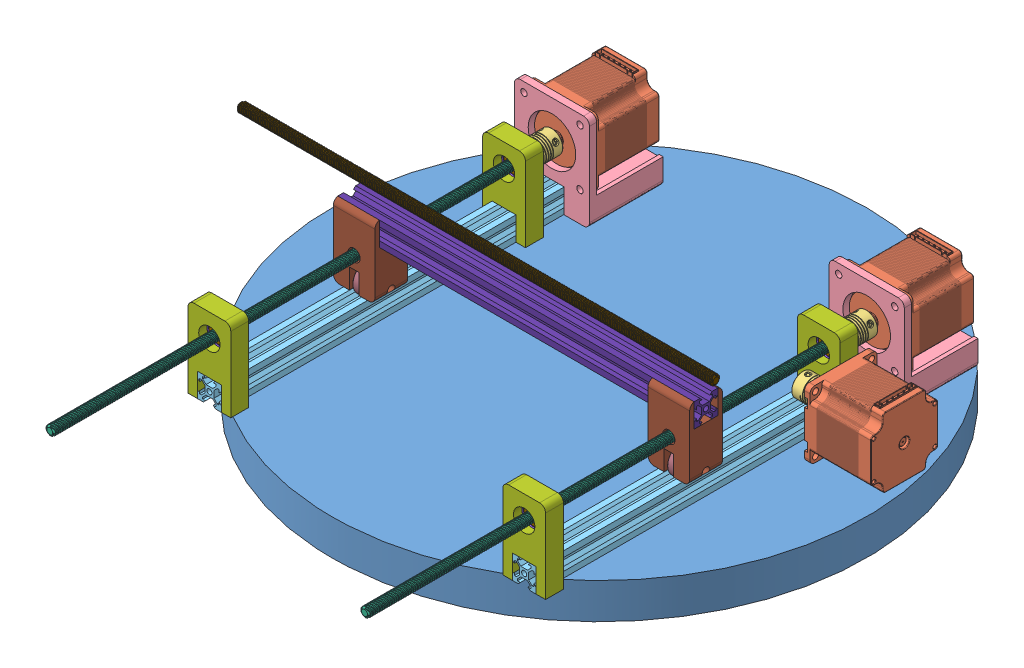
SolidWorks assembly EnsambleGeneral1, configuration Predeterminado. Lengths in mm.
Overall size (553.11 182.86 557.72).
58 component instances, 18 part files, 8 mates.
Components (placement in the parent):
- Base-1: Base [Predeterminado] at (-59.5476 49.1162 449.0688) size (450 30 450)
- EjeBase-1: EjeBase [Predeterminado] at (-180.3376 125.0022 256.2567) size (63.14 80.17 487.23)
  - Nema 23-1: Nema 23 [Default] at (-11.5289 2.714 38.3) size (56.4 59.4 76.6)
  - Coupler 6.35-8mm-1: Coupler 6.35-8mm [Default] at (-11.5289 2.714 113.0023) x (0.819898 0.57251 0) z (0 0 1) size (19.34 19.34 25)
  - SoporteNEMA-1-1: SoporteNEMA-1 [Predeterminado] at (12.0411 26.284 100.3) x (-1 0 0) z (0 0 -1) size (63.14 80.17 62)
  - BoschBase-1: BoschBase [Predeterminado] at (-21.6289 -25.886 38.3) size (20 20 350)
  - VarillaBase-1: VarillaBase [Default] at (-11.5289 2.714 522.6863) x (0.999103 -0.042354 0) z (0 0 1) size (8.33 8.33 405.47)
  - TopeVarilla-1: TopeVarilla [Predeterminado] at (-27.6485 -16.346 448.8) x (-1 0 0) z (0 0 -1) size (36 68 15)
    - SoporteVarilla1-1: SoporteVarilla1 [Predeterminado] at (-26.0197 -9.54 60.5) size (36 68 15)
    - skf_bearing_609_2-1: skf_bearing_609_2 [Default] at (-16.0197 19.06 74.5) x (0 0 -1) z (1 0 0) size (7 24 24)
      - skf_bearing_609_2_01-1: skf_bearing_609_2_01 [Default] at origin size (7 24 24)
      - skf_bearing_609_2_02-1: skf_bearing_609_2_02 [Default] at origin size (7 14.45 14.45)
      - skf_bearing_609_2_03-1: skf_bearing_609_2_03 [Default] at origin size (3.97 20.97 20.97)
  - TopeVarilla-2: TopeVarilla [Predeterminado] at (-27.6485 -16.346 201.0023) x (-1 0 0) z (0 0 -1) size (36 68 15)
    - SoporteVarilla1-1: SoporteVarilla1 [Predeterminado] at (-26.0197 -9.54 60.5) size (36 68 15)
    - skf_bearing_609_2-1: skf_bearing_609_2 [Default] at (-16.0197 19.06 74.5) x (0 0 -1) z (1 0 0) size (7 24 24)
      - skf_bearing_609_2_01-1: skf_bearing_609_2_01 [Default] at origin size (7 24 24)
      - skf_bearing_609_2_02-1: skf_bearing_609_2_02 [Default] at origin size (7 14.45 14.45)
      - skf_bearing_609_2_03-1: skf_bearing_609_2_03 [Default] at origin size (3.97 20.97 20.97)
- EjeBase-2: EjeBase [Predeterminado] at (84.3748 125.0022 256.2567) size (63.14 80.17 487.23)
  - Nema 23-1: Nema 23 [Default] at (-11.5289 2.714 38.3) size (56.4 59.4 76.6)
  - Coupler 6.35-8mm-1: Coupler 6.35-8mm [Default] at (-11.5289 2.714 113.0023) x (0.819898 0.57251 0) z (0 0 1) size (19.34 19.34 25)
  - SoporteNEMA-1-1: SoporteNEMA-1 [Predeterminado] at (12.0411 26.284 100.3) x (-1 0 0) z (0 0 -1) size (63.14 80.17 62)
  - BoschBase-1: BoschBase [Predeterminado] at (-21.6289 -25.886 38.3) size (20 20 350)
  - VarillaBase-1: VarillaBase [Default] at (-11.5289 2.714 522.6863) x (0.999103 -0.042354 0) z (0 0 1) size (8.33 8.33 405.47)
  - TopeVarilla-1: TopeVarilla [Predeterminado] at (-27.6485 -16.346 448.8) x (-1 0 0) z (0 0 -1) size (36 68 15)
    - SoporteVarilla1-1: SoporteVarilla1 [Predeterminado] at (-26.0197 -9.54 60.5) size (36 68 15)
    - skf_bearing_609_2-1: skf_bearing_609_2 [Default] at (-16.0197 19.06 74.5) x (0 0 -1) z (1 0 0) size (7 24 24)
      - skf_bearing_609_2_01-1: skf_bearing_609_2_01 [Default] at origin size (7 24 24)
      - skf_bearing_609_2_02-1: skf_bearing_609_2_02 [Default] at origin size (7 14.45 14.45)
      - skf_bearing_609_2_03-1: skf_bearing_609_2_03 [Default] at origin size (3.97 20.97 20.97)
  - TopeVarilla-2: TopeVarilla [Predeterminado] at (-27.6485 -16.346 201.0023) x (-1 0 0) z (0 0 -1) size (36 68 15)
    - SoporteVarilla1-1: SoporteVarilla1 [Predeterminado] at (-26.0197 -9.54 60.5) size (36 68 15)
    - skf_bearing_609_2-1: skf_bearing_609_2 [Default] at (-16.0197 19.06 74.5) x (0 0 -1) z (1 0 0) size (7 24 24)
      - skf_bearing_609_2_01-1: skf_bearing_609_2_01 [Default] at origin size (7 24 24)
      - skf_bearing_609_2_02-1: skf_bearing_609_2_02 [Default] at origin size (7 14.45 14.45)
      - skf_bearing_609_2_03-1: skf_bearing_609_2_03 [Default] at origin size (3.97 20.97 20.97)
- EjeY-1: EjeY [Predeterminado] at (-168.3529 121.4844 439.3712) size (553.11 140.41 56.4)
  - SoporteEjeY-1: SoporteEjeY [Predeterminado] at (-17.1016 3.702 20.9937) size (35 68.64 29.7)
    - SujeciónEjeY-1: SujeciónEjeY [Predeterminado] at (-24.012 20.0298 35) size (35 59.86 27.5)
    - T8-Screw-1: T8-Screw [Default] at (-6.512 2.5298 35) x (0 1 0) z (0 0 -1) size (22 22 16.4)
    - skf_bearing_61901_2-1: skf_bearing_61901_2 [Default] at (-9.4581 -20.8302 48.75) x (1 0 0) z (0 -0.067535 0.997717) size (6 24 24)
      - skf_bearing_61901_2_01-1: skf_bearing_61901_2_01 [Default] at origin size (6 24 24)
      - skf_bearing_61901_2_02-1: skf_bearing_61901_2_02 [Default] at origin size (6 16 16)
      - skf_bearing_61901_2_03-1: skf_bearing_61901_2_03 [Default] at origin size (3.18 21.18 20.29)
      - PiezaInterna-1: PiezaInterna [Predeterminado] x (0 0 -1) z (1 0 0) size (12 12 6)
  - SoporteEjeY-2: SoporteEjeY [Predeterminado] at (247.6084 3.702 20.9937) size (35 68.64 29.7)
    - SujeciónEjeY-1: SujeciónEjeY [Predeterminado] at (-24.012 20.0298 35) size (35 59.86 27.5)
    - T8-Screw-1: T8-Screw [Default] at (-6.512 2.5298 35) x (0 1 0) z (0 0 -1) size (22 22 16.4)
    - skf_bearing_61901_2-1: skf_bearing_61901_2 [Default] at (-9.4581 -20.8302 48.75) x (1 0 0) z (0 -0.067535 0.997717) size (6 24 24)
      - skf_bearing_61901_2_01-1: skf_bearing_61901_2_01 [Default] at origin size (6 24 24)
      - skf_bearing_61901_2_02-1: skf_bearing_61901_2_02 [Default] at origin size (6 16 16)
      - skf_bearing_61901_2_03-1: skf_bearing_61901_2_03 [Default] at origin size (3.18 21.18 20.29)
      - PiezaInterna-1: PiezaInterna [Predeterminado] x (0 0 -1) z (1 0 0) size (12 12 6)
  - BoschEjeY-1: BoschEjeY [Predeterminado] at (-41.1136 18.7318 79.7437) x (0 1 0) z (1 0 0) size (20 20 299.71)
  - VarillaEjeY-1: VarillaEjeY [Default] at (266.9965 53.3895 69.7725) x (0 -1 0) z (1 0 0) size (8.33 8.33 405.47)
  - Nema 23-1: Nema 23 [Default] at (417.4775 79.2944 61.7711) x (0 0 1) z (-1 0 0) size (56.4 59.4 76.6)
  - Coupler 6.35-8mm-1: Coupler 6.35-8mm [Default] at (344.5673 79.2944 61.7711) x (0 0 -1) z (1 0 0) size (19.34 19.34 25)
Mates (geometry in assembly coordinates):
- Coincidente1: coincident anti-aligned: plane of Base-1 through (-59.5476 79.1162 449.0688) normal (0 1 0); plane of EjeBase-1/SoporteNEMA-1-1 through (-168.2965 79.1162 294.5567) normal (0 -1 0)
- Coincidente2: coincident anti-aligned: plane of Base-1 through (-59.5476 79.1162 449.0688) normal (0 1 0); plane of EjeBase-2/SoporteNEMA-1-1 through (96.4159 79.1162 356.5567) normal (0 -1 0)
- Paralelo3: parallel aligned: plane of EjeBase-1/SoporteNEMA-1-1 through (-168.2965 151.2862 356.5567) normal (0 0 1); plane of EjeBase-2/SoporteNEMA-1-1 through (96.4159 151.2862 356.5567) normal (0 0 1)
- Coincidente5: coincident aligned: plane of EjeBase-1/SoporteNEMA-1-1 through (-168.2965 151.2862 356.5567) normal (0 0 1); plane of EjeBase-2/SoporteNEMA-1-1 through (96.4159 151.2862 356.5567) normal (0 0 1)
- Concéntrica1: concentric anti-aligned: cylinder of EjeBase-1/TopeVarilla-2/SoporteVarilla1-1 through (-191.9665 127.7162 389.7591) axis (0 0 1) radius 9; cylinder of EjeY-1/SoporteEjeY-1/SujeciónEjeY-1 through (-191.9665 127.7162 522.8649) axis (0 0 -1) radius 5.1
- Paralelo4: parallel anti-aligned: plane of EjeBase-1/BoschBase-1 through (-201.9665 99.1162 644.5567) normal (0 1 0); plane of EjeY-1/SoporteEjeY-1/SujeciónEjeY-1 through (-174.4665 100.3562 495.3649) normal (0 -1 0)
- Bloquear1: lock: unknown of Base-1; unknown of EjeBase-2/SoporteNEMA-1-1
- Bloquear2: lock: unknown of Base-1; unknown of EjeBase-1/SoporteNEMA-1-1
